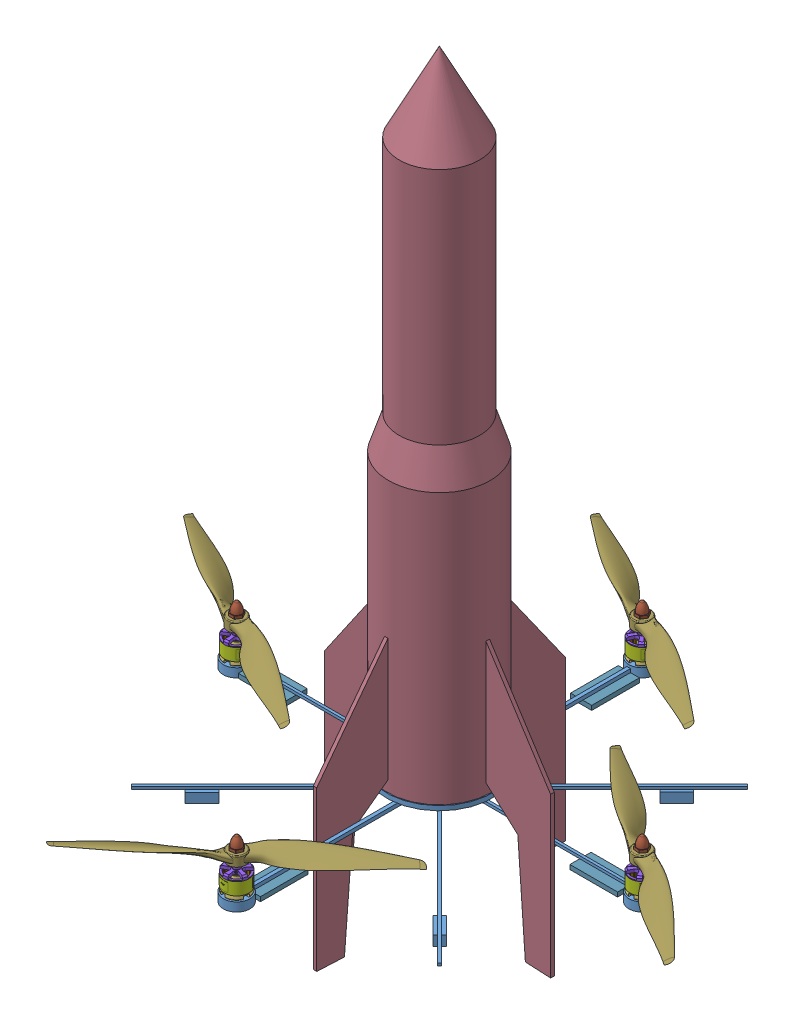
SolidWorks assembly Esamblaje Cohete, configuration Predeterminado. Lengths in mm.
Overall size (735.27 842.22 731.22).
107 component instances, 15 part files, 28 mates.
Components (placement in the parent):
- Base pila2.0-1: Base pila2.0 [Predeterminado] at (0.2487 0 -0.1681) x (0.339851 0 -0.940479) z (0.940479 0 0.339851) size (461.66 176.4 461.66)
- Batería-1: Batería [Predeterminado] at (-0.6009 5 2.1831) x (0.339851 0 -0.940479) z (0.940479 0 0.339851) size (45 125 28)
- Assembly-1: Assembly [Default] at (5.1808 -6.4568 -202.4162) x (-0.984129 0 0.177456) z (-0.177456 0 -0.984129) size (251.1 57.6 218.44)
  - Motor Casing-1: Motor Casing [Default] at (0.0476 0.0568 27.7) size (27.7 18.09 27.7)
  - Drive Shaft-1: Drive Shaft [Default] at (0.0476 25.2068 27.7) x (0 -1 0) z (-0.763091 0 -0.646291) size (26.25 3 3)
  - Electrical Windings-1: Electrical Windings [Default] at (0.0476 18.0568 27.7) x (1 0 -0.000785) z (-0.000785 0 -1) size (36.88 20.62 22) (hidden)
  - instrument ball bearing_68_iso-1: instrument ball bearing_68_iso [ISO 1224 - 390308 - R,8,DE,NC,8_68] at (0.0476 2.0568 27.7) x (0 -1 0) z (0.020466 0 0.999791) size (4 8 8)
  - e-ring external retaining ring_wti-4: e-ring external retaining ring_wti [Truarc X5133-14 - S0.14] at (0.0476 0.0355 27.7) x (0.994275 0 -0.106853) z (0 1 0) size (5.26 4.55 0.38)
  - Rotor Cover-1: Rotor Cover [Default] at (0.0476 5.0568 27.7) x (0.291228 0 -0.956654) z (0.956654 0 0.291228) size (27.65 14 28.06)
  - Rotor-1: Rotor [Default] at (0.0476 14.5568 27.7) x (-0.763091 0 -0.646291) z (0.646291 0 -0.763091) size (27.65 31.18 27.65)
  - Magnet-1: Magnet [Default] at (7.7444 12.0568 37.9586) x (0.799891 0 -0.600146) z (-0.600146 0 -0.799891) size (4 12 1.6)
  - Magnet-2: Magnet [Default] at (2.5312 12.0568 40.2822) x (0.98107 0 -0.193653) z (-0.193653 0 -0.98107) size (4 12 1.6)
  - Magnet-3: Magnet [Default] at (-3.174 12.0568 40.1138) x (0.967937 0 0.251195) z (0.251195 0 -0.967937) size (4 12 1.6)
  - Magnet-4: Magnet [Default] at (-8.2411 12.0568 37.4866) x (0.763091 0 0.646291) z (0.646291 0 -0.763091) size (4 12 1.6)
  - Magnet-5: Magnet [Default] at (-11.6666 12.0568 32.9211) x (0.407106 0 0.913381) z (0.913381 0 -0.407106) size (4 12 1.6)
  - Magnet-6: Magnet [Default] at (-12.7719 12.0568 27.3215) x (-0.029511 0 0.999564) z (0.999564 0 0.029511) size (4 12 1.6)
  - Magnet-7: Magnet [Default] at (-11.3381 12.0568 21.7969) x (-0.460283 0 0.887772) z (0.887772 0 0.460283) size (4 12 1.6)
  - Magnet-8: Magnet [Default] at (-7.6493 12.0568 17.4414) x (-0.799891 0 0.600146) z (0.600146 0 0.799891) size (4 12 1.6)
  - Magnet-9: Magnet [Default] at (-2.4361 12.0568 15.1178) x (-0.98107 0 0.193653) z (0.193653 0 0.98107) size (4 12 1.6)
  - Magnet-10: Magnet [Default] at (3.2691 12.0568 15.2862) x (-0.967937 0 -0.251195) z (-0.251195 0 0.967937) size (4 12 1.6)
  - Magnet-11: Magnet [Default] at (8.3362 12.0568 17.9134) x (-0.763091 0 -0.646291) z (-0.646291 0 0.763091) size (4 12 1.6)
  - Magnet-12: Magnet [Default] at (11.7617 12.0568 22.4789) x (-0.407106 0 -0.913381) z (-0.913381 0 0.407106) size (4 12 1.6)
  - Magnet-13: Magnet [Default] at (12.867 12.0568 28.0785) x (0.029511 0 -0.999564) z (-0.999564 0 -0.029511) size (4 12 1.6)
  - Magnet-14: Magnet [Default] at (11.4332 12.0568 33.6031) x (0.460283 0 -0.887772) z (-0.887772 0 -0.460283) size (4 12 1.6)
  - Stopper Screw-1: Stopper Screw [Default] at (-0.5987 21.8426 28.4631) x (-0.646291 0 0.763091) z (-0.763091 0 -0.646291) size (2.64 2.54 2.89)
  - Nut-2: Nut [Default] at (0.0983 41.5568 27.7396) x (-0.763091 0 -0.646291) z (0.646291 0 -0.763091) size (12.11 14.31 13.7)
  - APC 12x6-1: APC 12x6 [기본] at (0.0476 30.5568 27.7) x (-0.763091 0 -0.646291) z (0.646291 0 -0.763091) size (306.42 15.31 26.73)
- Assembly-2: Assembly [Default] at (231.7094 -6.4568 27.4322) x (-0.997612 0 0.069071) z (-0.069071 0 -0.997612) size (251.1 57.6 218.44)
  - Motor Casing-1: Motor Casing [Default] at (0.0476 0.0568 27.7) size (27.7 18.09 27.7)
  - Drive Shaft-1: Drive Shaft [Default] at (0.0476 25.2068 27.7) x (0 -1 0) z (-0.763091 0 -0.646291) size (26.25 3 3)
  - Electrical Windings-1: Electrical Windings [Default] at (0.0476 18.0568 27.7) x (1 0 -0.000785) z (-0.000785 0 -1) size (36.88 20.62 22) (hidden)
  - instrument ball bearing_68_iso-1: instrument ball bearing_68_iso [ISO 1224 - 390308 - R,8,DE,NC,8_68] at (0.0476 2.0568 27.7) x (0 -1 0) z (0.020466 0 0.999791) size (4 8 8)
  - e-ring external retaining ring_wti-4: e-ring external retaining ring_wti [Truarc X5133-14 - S0.14] at (0.0476 0.0355 27.7) x (0.994275 0 -0.106853) z (0 1 0) size (5.26 4.55 0.38)
  - Rotor Cover-1: Rotor Cover [Default] at (0.0476 5.0568 27.7) x (0.291228 0 -0.956654) z (0.956654 0 0.291228) size (27.65 14 28.06)
  - Rotor-1: Rotor [Default] at (0.0476 14.5568 27.7) x (-0.763091 0 -0.646291) z (0.646291 0 -0.763091) size (27.65 31.18 27.65)
  - Magnet-1: Magnet [Default] at (7.7444 12.0568 37.9586) x (0.799891 0 -0.600146) z (-0.600146 0 -0.799891) size (4 12 1.6)
  - Magnet-2: Magnet [Default] at (2.5312 12.0568 40.2822) x (0.98107 0 -0.193653) z (-0.193653 0 -0.98107) size (4 12 1.6)
  - Magnet-3: Magnet [Default] at (-3.174 12.0568 40.1138) x (0.967937 0 0.251195) z (0.251195 0 -0.967937) size (4 12 1.6)
  - Magnet-4: Magnet [Default] at (-8.2411 12.0568 37.4866) x (0.763091 0 0.646291) z (0.646291 0 -0.763091) size (4 12 1.6)
  - Magnet-5: Magnet [Default] at (-11.6666 12.0568 32.9211) x (0.407106 0 0.913381) z (0.913381 0 -0.407106) size (4 12 1.6)
  - Magnet-6: Magnet [Default] at (-12.7719 12.0568 27.3215) x (-0.029511 0 0.999564) z (0.999564 0 0.029511) size (4 12 1.6)
  - Magnet-7: Magnet [Default] at (-11.3381 12.0568 21.7969) x (-0.460283 0 0.887772) z (0.887772 0 0.460283) size (4 12 1.6)
  - Magnet-8: Magnet [Default] at (-7.6493 12.0568 17.4414) x (-0.799891 0 0.600146) z (0.600146 0 0.799891) size (4 12 1.6)
  - Magnet-9: Magnet [Default] at (-2.4361 12.0568 15.1178) x (-0.98107 0 0.193653) z (0.193653 0 0.98107) size (4 12 1.6)
  - Magnet-10: Magnet [Default] at (3.2691 12.0568 15.2862) x (-0.967937 0 -0.251195) z (-0.251195 0 0.967937) size (4 12 1.6)
  - Magnet-11: Magnet [Default] at (8.3362 12.0568 17.9134) x (-0.763091 0 -0.646291) z (-0.646291 0 0.763091) size (4 12 1.6)
  - Magnet-12: Magnet [Default] at (11.7617 12.0568 22.4789) x (-0.407106 0 -0.913381) z (-0.913381 0 0.407106) size (4 12 1.6)
  - Magnet-13: Magnet [Default] at (12.867 12.0568 28.0785) x (0.029511 0 -0.999564) z (-0.999564 0 -0.029511) size (4 12 1.6)
  - Magnet-14: Magnet [Default] at (11.4332 12.0568 33.6031) x (0.460283 0 -0.887772) z (-0.887772 0 -0.460283) size (4 12 1.6)
  - Stopper Screw-1: Stopper Screw [Default] at (-0.5987 21.8426 28.4631) x (-0.646291 0 0.763091) z (-0.763091 0 -0.646291) size (2.64 2.54 2.89)
  - Nut-2: Nut [Default] at (0.0983 41.5568 27.7396) x (-0.763091 0 -0.646291) z (0.646291 0 -0.763091) size (12.11 14.31 13.7)
  - APC 12x6-1: APC 12x6 [기본] at (0.0476 30.5568 27.7) x (-0.763091 0 -0.646291) z (0.646291 0 -0.763091) size (306.42 15.31 26.73)
- Assembly-3: Assembly [Default] at (-27.0171 -6.4568 224.6187) x (0.171843 0 -0.985124) z (0.985124 0 0.171843) size (251.1 57.6 218.44)
  - Motor Casing-1: Motor Casing [Default] at (0.0476 0.0568 27.7) size (27.7 18.09 27.7)
  - Drive Shaft-1: Drive Shaft [Default] at (0.0476 25.2068 27.7) x (0 -1 0) z (-0.763091 0 -0.646291) size (26.25 3 3)
  - Electrical Windings-1: Electrical Windings [Default] at (0.0476 18.0568 27.7) x (1 0 -0.000785) z (-0.000785 0 -1) size (36.88 20.62 22) (hidden)
  - instrument ball bearing_68_iso-1: instrument ball bearing_68_iso [ISO 1224 - 390308 - R,8,DE,NC,8_68] at (0.0476 2.0568 27.7) x (0 -1 0) z (0.020466 0 0.999791) size (4 8 8)
  - e-ring external retaining ring_wti-4: e-ring external retaining ring_wti [Truarc X5133-14 - S0.14] at (0.0476 0.0355 27.7) x (0.994275 0 -0.106853) z (0 1 0) size (5.26 4.55 0.38)
  - Rotor Cover-1: Rotor Cover [Default] at (0.0476 5.0568 27.7) x (0.291228 0 -0.956654) z (0.956654 0 0.291228) size (27.65 14 28.06)
  - Rotor-1: Rotor [Default] at (0.0476 14.5568 27.7) x (-0.763091 0 -0.646291) z (0.646291 0 -0.763091) size (27.65 31.18 27.65)
  - Magnet-1: Magnet [Default] at (7.7444 12.0568 37.9586) x (0.799891 0 -0.600146) z (-0.600146 0 -0.799891) size (4 12 1.6)
  - Magnet-2: Magnet [Default] at (2.5312 12.0568 40.2822) x (0.98107 0 -0.193653) z (-0.193653 0 -0.98107) size (4 12 1.6)
  - Magnet-3: Magnet [Default] at (-3.174 12.0568 40.1138) x (0.967937 0 0.251195) z (0.251195 0 -0.967937) size (4 12 1.6)
  - Magnet-4: Magnet [Default] at (-8.2411 12.0568 37.4866) x (0.763091 0 0.646291) z (0.646291 0 -0.763091) size (4 12 1.6)
  - Magnet-5: Magnet [Default] at (-11.6666 12.0568 32.9211) x (0.407106 0 0.913381) z (0.913381 0 -0.407106) size (4 12 1.6)
  - Magnet-6: Magnet [Default] at (-12.7719 12.0568 27.3215) x (-0.029511 0 0.999564) z (0.999564 0 0.029511) size (4 12 1.6)
  - Magnet-7: Magnet [Default] at (-11.3381 12.0568 21.7969) x (-0.460283 0 0.887772) z (0.887772 0 0.460283) size (4 12 1.6)
  - Magnet-8: Magnet [Default] at (-7.6493 12.0568 17.4414) x (-0.799891 0 0.600146) z (0.600146 0 0.799891) size (4 12 1.6)
  - Magnet-9: Magnet [Default] at (-2.4361 12.0568 15.1178) x (-0.98107 0 0.193653) z (0.193653 0 0.98107) size (4 12 1.6)
  - Magnet-10: Magnet [Default] at (3.2691 12.0568 15.2862) x (-0.967937 0 -0.251195) z (-0.251195 0 0.967937) size (4 12 1.6)
  - Magnet-11: Magnet [Default] at (8.3362 12.0568 17.9134) x (-0.763091 0 -0.646291) z (-0.646291 0 0.763091) size (4 12 1.6)
  - Magnet-12: Magnet [Default] at (11.7617 12.0568 22.4789) x (-0.407106 0 -0.913381) z (-0.913381 0 0.407106) size (4 12 1.6)
  - Magnet-13: Magnet [Default] at (12.867 12.0568 28.0785) x (0.029511 0 -0.999564) z (-0.999564 0 -0.029511) size (4 12 1.6)
  - Magnet-14: Magnet [Default] at (11.4332 12.0568 33.6031) x (0.460283 0 -0.887772) z (-0.887772 0 -0.460283) size (4 12 1.6)
  - Stopper Screw-1: Stopper Screw [Default] at (-0.5987 21.8426 28.4631) x (-0.646291 0 0.763091) z (-0.763091 0 -0.646291) size (2.64 2.54 2.89)
  - Nut-2: Nut [Default] at (0.0983 41.5568 27.7396) x (-0.763091 0 -0.646291) z (0.646291 0 -0.763091) size (12.11 14.31 13.7)
  - APC 12x6-1: APC 12x6 [기본] at (0.0476 30.5568 27.7) x (-0.763091 0 -0.646291) z (0.646291 0 -0.763091) size (306.42 15.31 26.73)
- Assembly-4: Assembly [Default] at (-234.3854 -6.4568 -27.3579) x (0.98299 0 -0.183659) z (0.183659 0 0.98299) size (251.1 57.6 218.44)
  - Motor Casing-1: Motor Casing [Default] at (0.0476 0.0568 27.7) size (27.7 18.09 27.7)
  - Drive Shaft-1: Drive Shaft [Default] at (0.0476 25.2068 27.7) x (0 -1 0) z (-0.763091 0 -0.646291) size (26.25 3 3)
  - Electrical Windings-1: Electrical Windings [Default] at (0.0476 18.0568 27.7) x (1 0 -0.000785) z (-0.000785 0 -1) size (36.88 20.62 22) (hidden)
  - instrument ball bearing_68_iso-1: instrument ball bearing_68_iso [ISO 1224 - 390308 - R,8,DE,NC,8_68] at (0.0476 2.0568 27.7) x (0 -1 0) z (0.020466 0 0.999791) size (4 8 8)
  - e-ring external retaining ring_wti-4: e-ring external retaining ring_wti [Truarc X5133-14 - S0.14] at (0.0476 0.0355 27.7) x (0.994275 0 -0.106853) z (0 1 0) size (5.26 4.55 0.38)
  - Rotor Cover-1: Rotor Cover [Default] at (0.0476 5.0568 27.7) x (0.291228 0 -0.956654) z (0.956654 0 0.291228) size (27.65 14 28.06)
  - Rotor-1: Rotor [Default] at (0.0476 14.5568 27.7) x (-0.763091 0 -0.646291) z (0.646291 0 -0.763091) size (27.65 31.18 27.65)
  - Magnet-1: Magnet [Default] at (7.7444 12.0568 37.9586) x (0.799891 0 -0.600146) z (-0.600146 0 -0.799891) size (4 12 1.6)
  - Magnet-2: Magnet [Default] at (2.5312 12.0568 40.2822) x (0.98107 0 -0.193653) z (-0.193653 0 -0.98107) size (4 12 1.6)
  - Magnet-3: Magnet [Default] at (-3.174 12.0568 40.1138) x (0.967937 0 0.251195) z (0.251195 0 -0.967937) size (4 12 1.6)
  - Magnet-4: Magnet [Default] at (-8.2411 12.0568 37.4866) x (0.763091 0 0.646291) z (0.646291 0 -0.763091) size (4 12 1.6)
  - Magnet-5: Magnet [Default] at (-11.6666 12.0568 32.9211) x (0.407106 0 0.913381) z (0.913381 0 -0.407106) size (4 12 1.6)
  - Magnet-6: Magnet [Default] at (-12.7719 12.0568 27.3215) x (-0.029511 0 0.999564) z (0.999564 0 0.029511) size (4 12 1.6)
  - Magnet-7: Magnet [Default] at (-11.3381 12.0568 21.7969) x (-0.460283 0 0.887772) z (0.887772 0 0.460283) size (4 12 1.6)
  - Magnet-8: Magnet [Default] at (-7.6493 12.0568 17.4414) x (-0.799891 0 0.600146) z (0.600146 0 0.799891) size (4 12 1.6)
  - Magnet-9: Magnet [Default] at (-2.4361 12.0568 15.1178) x (-0.98107 0 0.193653) z (0.193653 0 0.98107) size (4 12 1.6)
  - Magnet-10: Magnet [Default] at (3.2691 12.0568 15.2862) x (-0.967937 0 -0.251195) z (-0.251195 0 0.967937) size (4 12 1.6)
  - Magnet-11: Magnet [Default] at (8.3362 12.0568 17.9134) x (-0.763091 0 -0.646291) z (-0.646291 0 0.763091) size (4 12 1.6)
  - Magnet-12: Magnet [Default] at (11.7617 12.0568 22.4789) x (-0.407106 0 -0.913381) z (-0.913381 0 0.407106) size (4 12 1.6)
  - Magnet-13: Magnet [Default] at (12.867 12.0568 28.0785) x (0.029511 0 -0.999564) z (-0.999564 0 -0.029511) size (4 12 1.6)
  - Magnet-14: Magnet [Default] at (11.4332 12.0568 33.6031) x (0.460283 0 -0.887772) z (-0.887772 0 -0.460283) size (4 12 1.6)
  - Stopper Screw-1: Stopper Screw [Default] at (-0.5987 21.8426 28.4631) x (-0.646291 0 0.763091) z (-0.763091 0 -0.646291) size (2.64 2.54 2.89)
  - Nut-2: Nut [Default] at (0.0983 41.5568 27.7396) x (-0.763091 0 -0.646291) z (0.646291 0 -0.763091) size (12.11 14.31 13.7)
  - APC 12x6-1: APC 12x6 [기본] at (0.0476 30.5568 27.7) x (-0.763091 0 -0.646291) z (0.646291 0 -0.763091) size (306.42 15.31 26.73)
- Carcasa Cohete-1: Carcasa Cohete [Predeterminado] at (0.2487 0 -0.1681) x (-0.998857 0 -0.047808) z (0.047808 0 -0.998857) size (269 842.22 269)
- Driver-1: Driver [Predeterminado] at (187.7487 -8.4 0.6409) x (0 0 1) z (1 0 0) size (24 5 54)
- Driver-2: Driver [Predeterminado] at (0.2003 -18.4 187.3319) size (24 5 54)
- Driver-3: Driver [Predeterminado] at (-187.2513 -13.4 0.9124) x (0 0 -1) z (1 0 0) size (24 5 54)
- Driver-4: Driver [Predeterminado] at (0.1343 -18.4 -187.6681) size (24 5 54)
Mates (geometry in assembly coordinates):
- Coincidente1: coincident anti-aligned: plane of Base pila2.0-1 through (0.2487 5 -0.1681) normal (0 1 0); plane of Batería-1 through (-0.6009 5 2.1831) normal (0 -1 0)
- Coincidente2: coincident anti-aligned: plane of Base pila2.0-1 through (-12.918 75 -4.926) normal (0.940479 0 0.339851); plane of Batería-1 through (-6.121 130 -23.7356) normal (-0.940479 0 -0.339851)
- Coincidente3: coincident anti-aligned: plane of Base pila2.0-1 through (-8.2475 75 23.3439) normal (0.339851 0 -0.940479); plane of Batería-1 through (4.9192 130 28.1018) normal (-0.339851 0 0.940479)
- Concéntrica1: concentric anti-aligned: cylinder of Base pila2.0-1 through (0.2184 -16.4 -229.6681) axis (0 1 0) radius 15; cylinder of Assembly-1/Rotor Cover-1 through (0.2184 12.6 -229.6681) axis (0 -1 0) radius 13.825
- Coincidente4: coincident anti-aligned: plane of Base pila2.0-1 through (0.2184 -6.4 -229.6681) normal (0 1 0); plane of Assembly-1/Motor Casing-1 through (-11.9356 -6.4 -227.4765) normal (0 -1 0)
- Concéntrica2: concentric anti-aligned: cylinder of Base pila2.0-1 through (229.7487 -16.4 -0.1984) axis (0 1 0) radius 15; cylinder of Assembly-2/Rotor Cover-1 through (229.7487 12.6 -0.1984) axis (0 -1 0) radius 13.825
- Coincidente5: coincident anti-aligned: plane of Base pila2.0-1 through (229.7487 -6.4 -0.1984) normal (0 1 0); plane of Assembly-2/Motor Casing-1 through (217.4282 -6.4 0.6546) normal (0 -1 0)
- Concéntrica3: concentric anti-aligned: cylinder of Assembly-3/Rotor Cover-1 through (0.279 12.6 229.3319) axis (0 -1 0) radius 13.825; cylinder of Base pila2.0-1 through (0.279 -16.4 229.3319) axis (0 1 0) radius 15
- Coincidente6: coincident anti-aligned: plane of Base pila2.0-1 through (0.279 -6.4 229.3319) normal (0 1 0); plane of Assembly-3/Motor Casing-1 through (2.4013 -6.4 217.1656) normal (0 -1 0)
- Concéntrica4: concentric anti-aligned: cylinder of Base pila2.0-1 through (-229.2513 -16.4 -0.1378) axis (0 1 0) radius 15; cylinder of Assembly-4/Rotor Cover-1 through (-229.2513 12.6 -0.1378) axis (0 -1 0) radius 13.825
- Coincidente7: coincident anti-aligned: plane of Base pila2.0-1 through (-229.2513 -6.4 -0.1378) normal (0 1 0); plane of Assembly-4/Motor Casing-1 through (-217.1113 -6.4 -2.406) normal (0 -1 0)
- Concéntrica6: concentric aligned: cylinder of Base pila2.0-1 through (0.2487 0 -0.1681) axis (0 -1 0) radius 59; cylinder of Carcasa Cohete-1 through (0.2487 310 -0.1681) axis (0 -1 0) radius 53.5
- Coincidente31: coincident anti-aligned: plane of Base pila2.0-1 through (0.2487 0 -0.1681) normal (0 1 0); plane of Carcasa Cohete-1 through (0.2487 0 -0.1681) normal (0 -1 0)
- Coincidente32: coincident aligned: plane of Base pila2.0-1 through (0.2487 0 -0.1681) normal (0 1 0)
- Coincidente33: coincident aligned: plane of Base pila2.0-1 through (0.2487 0 0) normal (0 0 1)
- Coincidente34: coincident aligned: plane of Base pila2.0-1 through (0 0 -0.1681) normal (1 0 0)
- Coincidente35: coincident anti-aligned: plane of Base pila2.0-1 through (214.7487 -8.4 1.5) normal (0 -1 0); plane of Driver-1 through (187.7487 -8.4 0.6409) normal (0 1 0)
- Paralelo11: parallel aligned: plane of Base pila2.0-1 through (214.7487 -5.4 -1.5) normal (0 0 -1); plane of Driver-1 through (214.7487 -13.4 -11.3591) normal (0 0 -1)
- Tangente1: tangent anti-aligned: cylinder of Base pila2.0-1 through (229.7487 -16.4 -0.1984) axis (0 1 0) radius 15; plane of Driver-1 through (214.7487 -13.4 12.6409) normal (1 0 0)
- Coincidente40: coincident anti-aligned: plane of Base pila2.0-1 through (-2 -13.4 214.3319) normal (0 -1 0); plane of Driver-2 through (0.2003 -13.4 187.3319) normal (0 1 0)
- Tangente3: tangent anti-aligned: cylinder of Base pila2.0-1 through (0.279 -16.4 229.3319) axis (0 1 0) radius 15; plane of Driver-2 through (12.2003 -13.4 214.3319) normal (0 0 1)
- Paralelo13: parallel aligned: plane of Base pila2.0-1 through (-2 -9.4 214.3319) normal (-1 0 0); plane of Driver-2 through (-11.7997 -13.4 214.3319) normal (-1 0 0)
- Coincidente42: coincident anti-aligned: plane of Base pila2.0-1 through (-214.2513 -8.4 1.5) normal (0 -1 0); plane of Driver-3 through (-187.2513 -8.4 0.9124) normal (0 1 0)
- Tangente4: tangent anti-aligned: cylinder of Base pila2.0-1 through (-229.2513 -16.4 -0.1378) axis (0 1 0) radius 15; plane of Driver-3 through (-214.2513 -8.4 -11.0876) normal (-1 0 0)
- Paralelo14: parallel aligned: plane of Base pila2.0-1 through (-214.2513 -5.4 1.5) normal (0 0 1); plane of Driver-3 through (-160.2513 -8.4 12.9124) normal (0 0 1)
- Coincidente44: coincident anti-aligned: plane of Base pila2.0-1 through (-2 -13.4 -214.6681) normal (0 -1 0); plane of Driver-4 through (0.1343 -13.4 -187.6681) normal (0 1 0)
- Tangente5: tangent anti-aligned: cylinder of Base pila2.0-1 through (0.2184 -16.4 -229.6681) axis (0 1 0) radius 15; plane of Driver-4 through (12.1343 -13.4 -214.6681) normal (0 0 -1)
- Paralelo15: parallel aligned: plane of Base pila2.0-1 through (-2 -9.4 -214.6681) normal (-1 0 0); plane of Driver-4 through (-11.8657 -13.4 -160.6681) normal (-1 0 0)
